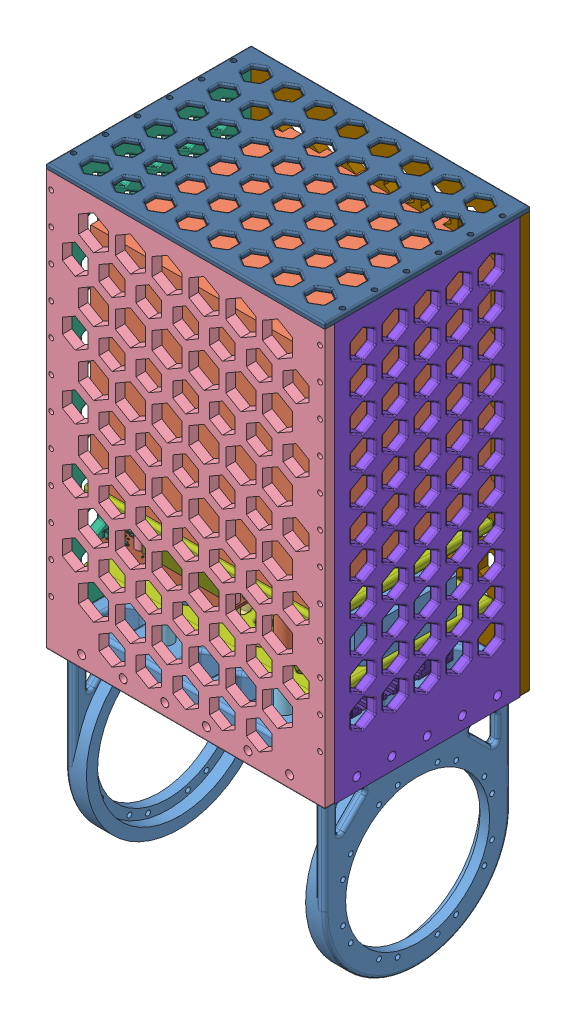
SolidWorks assembly upperbody, configuration 默认. Lengths in mm. (continued)
Components (placement in the parent): (continued)
- 交换机-1: 交换机 [默认] at (61.0275 78.8383 258.5616) x (0 0 1) z (0 -1 0) size (65.92 49.68 16.5)
  - LX-SWF502-2.step-1: LX-SWF502-2.step [Default] at (-129.5338 -11.9883 -6.5513) size (65.92 49.68 16.5)
    - RJEO-D19.step-1: RJEO-D19.step [Default] at (21.7657 41.0001 1.6) size (1.62 0.82 0.56)
      - LED0603N.step-1: LED0603N.step [Default] at origin size (1.62 0.82 0.56)
        - COMPOUND.step-1: COMPOUND.step [Default] at origin size (1.62 0.82 0.56)
    - RJEO-D2.step-1: RJEO-D2.step [Default] at (30.6411 41.0001 1.6) size (1.62 0.82 0.56)
      - LED0603N.step-1: LED0603N.step [Default] at origin size (1.62 0.82 0.56)
        - COMPOUND.step-1: COMPOUND.step [Default] at origin size (1.62 0.82 0.56)
    - RJEO-D20.step-1: RJEO-D20.step [Default] at (44.1334 41.0001 1.6) size (1.62 0.82 0.56)
      - LED0603N.step-1: LED0603N.step [Default] at origin size (1.62 0.82 0.56)
        - COMPOUND.step-1: COMPOUND.step [Default] at origin size (1.62 0.82 0.56)
    - RJEO-D21.step-1: RJEO-D21.step [Default] at (39.6501 41.0001 1.6) size (1.62 0.82 0.56)
      - LED0603N.step-1: LED0603N.step [Default] at origin size (1.62 0.82 0.56)
        - COMPOUND.step-1: COMPOUND.step [Default] at origin size (1.62 0.82 0.56)
    - RJEO-D22.step-1: RJEO-D22.step [Default] at (35.1271 41.0001 1.6) size (1.62 0.82 0.56)
      - LED0603N.step-1: LED0603N.step [Default] at origin size (1.62 0.82 0.56)
        - COMPOUND.step-1: COMPOUND.step [Default] at origin size (1.62 0.82 0.56)
    - RJEO-D1.step-1: RJEO-D1.step [Default] at (26.2147 41.0001 1.6) size (1.62 0.82 0.56)
      - LED0603N.step-1: LED0603N.step [Default] at origin size (1.62 0.82 0.56)
        - COMPOUND.step-1: COMPOUND.step [Default] at origin size (1.62 0.82 0.56)
    - RJEO-C10.step-1: RJEO-C10.step [Default] at (28.0001 37.4021 1.6) x (0 1 0) z (0 0 1) size (1 0.5 0.5)
      - 0402.step-1: 0402.step [Default] at origin size (1 0.5 0.5)
        - SOLID.step-1: SOLID.step [Default] at origin size (1 0.5 0.5)
    - RJEO-C11.step-1: RJEO-C11.step [Default] at (22.346 36.1431 1.6) x (-1 0 0) z (0 0 1) size (1 0.5 0.5)
      - 0402.step-1: 0402.step [Default] at origin size (1 0.5 0.5)
        - SOLID.step-1: SOLID.step [Default] at origin size (1 0.5 0.5)
    - RJEO-C13.step-1: RJEO-C13.step [Default] at (28.1391 26.6451 1.6) x (0 -1 0) z (0 0 1) size (1 0.5 0.5)
      - 0402.step-1: 0402.step [Default] at origin size (1 0.5 0.5)
        - SOLID.step-1: SOLID.step [Default] at origin size (1 0.5 0.5)
    - RJEO-C14.step-1: RJEO-C14.step [Default] at (32.6271 28.0611 1.6) x (0 -1 0) z (0 0 1) size (1 0.5 0.5)
      - 0402-1.step-1: 0402-1.step [Default] at origin size (1 0.5 0.5)
        - SOLID-0.step-1: SOLID-0.step [Default] at origin size (1 0.5 0.5)
    - RJEO-C15.step-1: RJEO-C15.step [Default] at (33.7611 35.9131 1.6) size (1 0.5 0.5)
      - 0402.step-1: 0402.step [Default] at origin size (1 0.5 0.5)
        - SOLID.step-1: SOLID.step [Default] at origin size (1 0.5 0.5)
    - RJEO-C16.step-1: RJEO-C16.step [Default] at (25.0001 37.5751 1.6) x (0 1 0) z (0 0 1) size (1 0.5 0.5)
      - 0402.step-1: 0402.step [Default] at origin size (1 0.5 0.5)
        - SOLID.step-1: SOLID.step [Default] at origin size (1 0.5 0.5)
    - RJEO-C17.step-1: RJEO-C17.step [Default] at (21.666 30.3191 1.6) x (-0.707107 -0.707107 0) z (0 0 1) size (1 0.5 0.5)
      - 0402.step-1: 0402.step [Default] at origin size (1 0.5 0.5)
        - SOLID.step-1: SOLID.step [Default] at origin size (1 0.5 0.5)
    - RJEO-C18.step-1: RJEO-C18.step [Default] at (23.917 26.8671 1.6) x (-0.707107 -0.707107 0) z (0 0 1) size (1 0.5 0.5)
      - 0402.step-1: 0402.step [Default] at origin size (1 0.5 0.5)
        - SOLID.step-1: SOLID.step [Default] at origin size (1 0.5 0.5)
    - RJEO-C19.step-1: RJEO-C19.step [Default] at (34.9891 39.2441 1.6) size (1 0.5 0.5)
      - 0402.step-1: 0402.step [Default] at origin size (1 0.5 0.5)
        - SOLID.step-1: SOLID.step [Default] at origin size (1 0.5 0.5)
    - RJEO-C2.step-1: RJEO-C2.step [Default] at (32.8971 20.6 1.6) x (0 1 0) z (0 0 1) size (1 0.5 0.5)
      - 0402.step-1: 0402.step [Default] at origin size (1 0.5 0.5)
        - SOLID.step-1: SOLID.step [Default] at origin size (1 0.5 0.5)
    - RJEO-C20.step-1: RJEO-C20.step [Default] at (31.5481 20.6 1.6) x (0 1 0) z (0 0 1) size (1 0.5 0.5)
      - 0402.step-1: 0402.step [Default] at origin size (1 0.5 0.5)
        - SOLID.step-1: SOLID.step [Default] at origin size (1 0.5 0.5)
    - RJEO-C25.step-1: RJEO-C25.step [Default] at (13.815 20.6 1.6) x (0 1 0) z (0 0 1) size (1 0.5 0.5)
      - 0402.step-1: 0402.step [Default] at origin size (1 0.5 0.5)
        - SOLID.step-1: SOLID.step [Default] at origin size (1 0.5 0.5)
    - RJEO-C37.step-1: RJEO-C37.step [Default] at (23.177 27.5921 1.6) x (-0.707107 -0.707107 0) z (0 0 1) size (1 0.5 0.5)
      - 0402.step-1: 0402.step [Default] at origin size (1 0.5 0.5)
        - SOLID.step-1: SOLID.step [Default] at origin size (1 0.5 0.5)
    - RJEO-C7.step-1: RJEO-C7.step [Default] at (34.7321 30.7291 1.6) x (0 -1 0) z (0 0 1) size (1 0.5 0.5)
      - 0402.step-1: 0402.step [Default] at origin size (1 0.5 0.5)
        - SOLID.step-1: SOLID.step [Default] at origin size (1 0.5 0.5)
    - RJEO-C8.step-1: RJEO-C8.step [Default] at (29.1961 26.6451 1.6) x (0 -1 0) z (0 0 1) size (1 0.5 0.5)
      - 0402.step-1: 0402.step [Default] at origin size (1 0.5 0.5)
        - SOLID.step-1: SOLID.step [Default] at origin size (1 0.5 0.5)
    - RJEO-C21.step-1: RJEO-C21.step [Default] at (5.908 27.1321 1.6) x (-1 0 0) z (0 0 1) size (1 0.5 0.5)
      - C0402.step-1: C0402.step [Default] at origin size (1 0.5 0.5)
        - SOLID-1.step-1: SOLID-1.step [Default] at origin size (1 0.5 0.5)
    - RJEO-C22.step-1: RJEO-C22.step [Default] at (6.552 21.19 1.6) size (1 0.5 0.5)
      - C0402.step-1: C0402.step [Default] at origin size (1 0.5 0.5)
        - SOLID-1.step-1: SOLID-1.step [Default] at origin size (1 0.5 0.5)
    - RJEO-C3.step-1: RJEO-C3.step [Default] at (32.5331 37.9101 1.6) x (0 1 0) z (0 0 1) size (1 0.5 0.5)
      - C0402.step-1: C0402.step [Default] at origin size (1 0.5 0.5)
        - SOLID-1.step-1: SOLID-1.step [Default] at origin size (1 0.5 0.5)
    - RJEO-C4.step-1: RJEO-C4.step [Default] at (18.817 32.7271 1.6) x (-1 0 0) z (0 0 1) size (1 0.5 0.5)
      - C0402.step-1: C0402.step [Default] at origin size (1 0.5 0.5)
        - SOLID-1.step-1: SOLID-1.step [Default] at origin size (1 0.5 0.5)
    - RJEO-C5.step-1: RJEO-C5.step [Default] at (18.81 37.8231 1.6) x (-1 0 0) z (0 0 1) size (1 0.5 0.5)
      - C0402.step-1: C0402.step [Default] at origin size (1 0.5 0.5)
        - SOLID-1.step-1: SOLID-1.step [Default] at origin size (1 0.5 0.5)
    - RJEO-C1.step-1: RJEO-C1.step [Default] at (51.3311 20.6 1.6) x (0 1 0) z (0 0 1) size (1 0.5 0.5)
      - 0402.step-1: 0402.step [Default] at origin size (1 0.5 0.5)
        - SOLID.step-1: SOLID.step [Default] at origin size (1 0.5 0.5)
    - RJEO-R11.step-1: RJEO-R11.step [Default] at (6.402 25.9921 1.6) x (-1 0 0) z (0 0 1) size (1 0.5 0.5)
      - 0402-2.step-1: 0402-2.step [Default] at origin size (1 0.5 0.5)
        - SOLID-2.step-1: SOLID-2.step [Default] at origin size (1 0.5 0.5)
    - RJEO-R12.step-1: RJEO-R12.step [Default] at (3.948 21.19 1.6) size (1 0.5 0.5)
      - 0402-2.step-1: 0402-2.step [Default] at origin size (1 0.5 0.5)
        - SOLID-2.step-1: SOLID-2.step [Default] at origin size (1 0.5 0.5)
    - RJEO-R13.step-1: RJEO-R13.step [Default] at (1.211 22.273 1.6) x (0 -1 0) z (0 0 1) size (1 0.5 0.5)
      - 0402-2.step-1: 0402-2.step [Default] at origin size (1 0.5 0.5)
        - SOLID-2.step-1: SOLID-2.step [Default] at origin size (1 0.5 0.5)
    - RJEO-R14.step-1: RJEO-R14.step [Default] at (2.295 24.326 1.6) x (0 -1 0) z (0 0 1) size (1 0.5 0.5)
      - 0402-2.step-1: 0402-2.step [Default] at origin size (1 0.5 0.5)
        - SOLID-2.step-1: SOLID-2.step [Default] at origin size (1 0.5 0.5)
    - RJEO-R15.step-1: RJEO-R15.step [Default] at (2.295 21.285 1.6) x (0 1 0) z (0 0 1) size (1 0.5 0.5)
      - 0402-2.step-1: 0402-2.step [Default] at origin size (1 0.5 0.5)
        - SOLID-2.step-1: SOLID-2.step [Default] at origin size (1 0.5 0.5)
    - RJEO-R2.step-1: RJEO-R2.step [Default] at (20.272 31.5191 1.6) size (1 0.5 0.5)
      - 0402-2.step-1: 0402-2.step [Default] at origin size (1 0.5 0.5)
        - SOLID-2.step-1: SOLID-2.step [Default] at origin size (1 0.5 0.5)
    - RJEO-R20.step-1: RJEO-R20.step [Default] at (26.4001 42.3001 1.6) size (1 0.5 0.5)
      - 0402-2.step-1: 0402-2.step [Default] at origin size (1 0.5 0.5)
        - SOLID-2.step-1: SOLID-2.step [Default] at origin size (1 0.5 0.5)
    - RJEO-R21.step-1: RJEO-R21.step [Default] at (31.0661 42.3001 1.6) size (1 0.5 0.5)
      - 0402-2.step-1: 0402-2.step [Default] at origin size (1 0.5 0.5)
        - SOLID-2.step-1: SOLID-2.step [Default] at origin size (1 0.5 0.5)
    - RJEO-R22.step-1: RJEO-R22.step [Default] at (35.6971 42.3001 1.6) size (1 0.5 0.5)
      - 0402-2.step-1: 0402-2.step [Default] at origin size (1 0.5 0.5)
        - SOLID-2.step-1: SOLID-2.step [Default] at origin size (1 0.5 0.5)
    - RJEO-R23.step-1: RJEO-R23.step [Default] at (40.2871 42.3001 1.6) size (1 0.5 0.5)
      - 0402-2.step-1: 0402-2.step [Default] at origin size (1 0.5 0.5)
        - SOLID-2.step-1: SOLID-2.step [Default] at origin size (1 0.5 0.5)
    - RJEO-R24.step-1: RJEO-R24.step [Default] at (45.0261 42.3001 1.6) size (1 0.5 0.5)
      - 0402-2.step-1: 0402-2.step [Default] at origin size (1 0.5 0.5)
        - SOLID-2.step-1: SOLID-2.step [Default] at origin size (1 0.5 0.5)
    - RJEO-R26.step-1: RJEO-R26.step [Default] at (21.524 42.3001 1.6) size (1 0.5 0.5)
      - 0402-2.step-1: 0402-2.step [Default] at origin size (1 0.5 0.5)
        - SOLID-2.step-1: SOLID-2.step [Default] at origin size (1 0.5 0.5)
    - RJEO-R3.step-1: RJEO-R3.step [Default] at (33.6221 38.4311 1.6) x (0 -1 0) z (0 0 1) size (1 0.5 0.5)
      - 0402-2.step-1: 0402-2.step [Default] at origin size (1 0.5 0.5)
        - SOLID-2.step-1: SOLID-2.step [Default] at origin size (1 0.5 0.5)
    - RJEO-R4.step-1: RJEO-R4.step [Default] at (30.3291 38.4071 1.6) x (0 -1 0) z (0 0 1) size (1 0.5 0.5)
      - 0402-2.step-1: 0402-2.step [Default] at origin size (1 0.5 0.5)
        - SOLID-2.step-1: SOLID-2.step [Default] at origin size (1 0.5 0.5)
    - RJEO-R5.step-1: RJEO-R5.step [Default] at (44.0581 42.3001 1.6) x (-1 0 0) z (0 0 1) size (1 0.5 0.5)
      - 0402-2.step-1: 0402-2.step [Default] at origin size (1 0.5 0.5)
        - SOLID-2.step-1: SOLID-2.step [Default] at origin size (1 0.5 0.5)
    - RJEO-R6.step-1: RJEO-R6.step [Default] at (39.2791 42.3001 1.6) x (-1 0 0) z (0 0 1) size (1 0.5 0.5)
      - 0402-2.step-1: 0402-2.step [Default] at origin size (1 0.5 0.5)
        - SOLID-2.step-1: SOLID-2.step [Default] at origin size (1 0.5 0.5)
    - RJEO-R7.step-1: RJEO-R7.step [Default] at (34.6091 42.3001 1.6) x (-1 0 0) z (0 0 1) size (1 0.5 0.5)
      - 0402-2.step-1: 0402-2.step [Default] at origin size (1 0.5 0.5)
        - SOLID-2.step-1: SOLID-2.step [Default] at origin size (1 0.5 0.5)
    - RJEO-R8.step-1: RJEO-R8.step [Default] at (30.0421 42.3001 1.6) x (-1 0 0) z (0 0 1) size (1 0.5 0.5)
      - 0402-2.step-1: 0402-2.step [Default] at origin size (1 0.5 0.5)
        - SOLID-2.step-1: SOLID-2.step [Default] at origin size (1 0.5 0.5)
    - RJEO-R9.step-1: RJEO-R9.step [Default] at (25.3031 42.3001 1.6) x (-1 0 0) z (0 0 1) size (1 0.5 0.5)
      - 0402-2.step-1: 0402-2.step [Default] at origin size (1 0.5 0.5)
        - SOLID-2.step-1: SOLID-2.step [Default] at origin size (1 0.5 0.5)
    - RJEO-R1.step-1: RJEO-R1.step [Default] at (31.4191 37.4141 1.6) x (0 1 0) z (0 0 1) size (1 0.5 0.5)
      - 0402-2.step-1: 0402-2.step [Default] at origin size (1 0.5 0.5)
        - SOLID-2.step-1: SOLID-2.step [Default] at origin size (1 0.5 0.5)
    - RJEO-JP1.step-1: RJEO-JP1.step [Default] at (12.001 40.0001 1.6) x (-1 0 0) z (0 0 1) size (7.5 5.9 10.6)
      - SIP2.step-1: SIP2.step [Default] at origin size (7.5 5.9 10.6)
        - COMPOUND-3.step-1: COMPOUND-3.step [Default] at origin size (7.5 5.9 10.6)
    - RJEO-DXFRM3.step-1: RJEO-DXFRM3.step [Default] at (21.989 19.3 1.6) x (-1 0 0) z (0 0 1) size (15.1 10 4.5)
      - NS892407B.step-1: NS892407B.step [Default] at origin size (15.1 10 4.5)
        - COMPOUND-4.step-1: COMPOUND-4.step [Default] at origin size (15.1 10 4.5)
    - RJEO-DXFRM1.step-1: RJEO-DXFRM1.step [Default] at (41.7141 19.3 1.6) x (-1 0 0) z (0 0 1) size (15.1 10 4.5)
      - NS892407B.step-1: NS892407B.step [Default] at origin size (15.1 10 4.5)
        - COMPOUND-4.step-1: COMPOUND-4.step [Default] at origin size (15.1 10 4.5)
    - RJEO-L2.step-1: RJEO-L2.step [Default] at (10.114 25.031 1.6) x (0 -1 0) z (0 0 1) size (4.4 4.2 2.1)
      - L10A.step-1: L10A.step [Default] at origin size (4.4 4.2 2.1)
        - SOLID-5.step-1: SOLID-5.step [Default] at origin size (4.4 4.2 2.1)
    - RJEO-TC4.step-1: RJEO-TC4.step [Default] at (4.629 32.6291 1.6) x (0 -1 0) z (0 0 1) size (6.6 7.8 7.75)
      - CAP-E-SMD-D6.3.step-1: CAP-E-SMD-D6.3.step [Default] at origin size (6.6 7.8 7.75)
        - SOLID-6.step-1: SOLID-6.step [Default] at origin size (6.6 7.8 7.75)
    - RJEO-TC1.step-1: RJEO-TC1.step [Default] at (16 28.8001 1.6) x (0 1 0) z (0 0 1) size (6.6 7.8 7.75)
      - CAP-E-SMD-D6.3.step-1: CAP-E-SMD-D6.3.step [Default] at origin size (6.6 7.8 7.75)
        - SOLID-6.step-1: SOLID-6.step [Default] at origin size (6.6 7.8 7.75)
    - RJEO-TRS1.step-1: RJEO-TRS1.step [Default] at (41.5201 33.5001 1.6) x (0 -1 0) z (0 0 1) size (12.7 9.5 5.95)
      - RJ45-8PIN.step-1: RJ45-8PIN.step [Default] at origin size (12.7 9.5 5.95)
        - COMPOUND-7.step-1: COMPOUND-7.step [Default] at origin size (12.7 9.5 5.95)
    - RJEO-Y6.step-1: RJEO-Y6.step [Default] at (18.772 35.3521 1.6) x (0 1 0) z (0 0 1) size (3.2 2.5 0.72)
      - SM091.step-1: SM091.step [Default] at origin size (3.2 2.5 0.72)
        - SOLID-8.step-1: SOLID-8.step [Default] at origin size (3.2 2.5 0.72)
    - RJEO-U1.step-1: RJEO-U1.step [Default] at (6.457 22.482 1.6) x (0 1 0) z (0 0 1) size (2.88 2.79 1.64)
      - SOT23-6.step-1: SOT23-6.step [Default] at origin size (2.88 2.79 1.64)
        - COMPOUND-9.step-1: COMPOUND-9.step [Default] at origin size (2.88 2.79 1.64)
    - RJEO-U2.step-1: RJEO-U2.step [Default] at (28.0001 32.0001 1.6) x (-1 0 0) z (0 0 1) size (6 6 0.85)
      - QFN48_04_EPAD.step-1: QFN48_04_EPAD.step [Default] at origin size (6 6 0.85)
        - COMPOUND-10.step-1: COMPOUND-10.step [Default] at origin size (6 6 0.85)
    - RJEO-H6.step-1: RJEO-H6.step [Default] at (56.8961 40.8691 1.6) x (-1 0 0) z (0 0 1) size (16.45 16.05 15.8)
      - RJ45-1X1-B.step-1: RJ45-1X1-B.step [Default] at origin size (16.45 16.05 15.8)
        - COMPOUND-11.step-1: COMPOUND-11.step [Default] at origin size (16.45 16.05 15.8)
    - RJEO-H7.step-1: RJEO-H7.step [Default] at (33.1521 2.093 1.6) size (63.76 15.76 16.2)
      - RJ45-1X4-B.step-1: RJ45-1X4-B.step [Default] at origin size (63.76 15.76 16.2)
        - COMPOUND-12.step-1: COMPOUND-12.step [Default] at origin size (63.76 15.76 16.2)
    - Board.step-1: Board.step [Default] at origin size (65.92 43.41 1.6)
- 转压-1: 转压 [默认] at (54.0084 99.9888 161.9625) x (-1 0 0) z (0 0 -1) size (57.6 22 63.7)
- ctrlbox-3: ctrlbox [默认] at (5.0084 130.5588 162) size (148 6 110)
- M6螺柱35-3: M6螺柱35 [默认] at (42.5084 93.9888 122) x (0.932693 0 -0.360672) z (0.360672 0 0.932693) size (10 35 10)
- M6螺柱35-4: M6螺柱35 [默认] at (42.5084 93.9888 202) x (0.513313 0 -0.858202) z (0.858202 0 0.513313) size (10 35 10)
- M3螺柱10-5: M3螺柱10 [默认] at (10.5084 93.9888 116) size (6 10 6)
- M3螺柱10-6: M3螺柱10 [默认] at (-47.4916 93.9888 116) size (6 10 6)
- M3螺柱10-7: M3螺柱10 [默认] at (-47.4916 93.9888 202) size (6 10 6)
- M3螺柱10-8: M3螺柱10 [默认] at (10.5084 93.9888 202) size (6 10 6)
- M3螺柱25-1: M3螺柱25 [默认] at (10.5084 105.5588 116) x (0.994103 0 0.108442) z (-0.108442 0 0.994103) size (6 25 6)
- M3螺柱25-2: M3螺柱25 [默认] at (-47.4916 105.5588 116) x (0.999732 0 0.023161) z (-0.023161 0 0.999732) size (6 25 6)
- M3螺柱25-3: M3螺柱25 [默认] at (-47.4916 105.5588 202) x (0.999732 0 0.023161) z (-0.023161 0 0.999732) size (6 25 6)
- M3螺柱25-4: M3螺柱25 [默认] at (10.5084 105.5588 202) x (0.999732 0 0.023161) z (-0.023161 0 0.999732) size (6 25 6)
- M4螺柱6-1: M4螺柱6 [默认] at (51.5084 93.9888 188.9625) x (0.999997 0 -0.002414) z (0.002414 0 0.999997) size (6 6 6)
- M4螺柱6-2: M4螺柱6 [默认] at (51.5084 93.9888 134.9625) x (0.9996 0 -0.02829) z (0.02829 0 0.9996) size (6 6 6)
Mates (geometry in assembly coordinates):
- Coincident1: coincident anti-aligned: plane of crotch-1 through (85.5084 62.9888 162) normal (0 1 0); plane of imu-1 through (4.5084 62.9888 136) normal (0 -1 0)
- Concentric1: concentric anti-aligned: cylinder of crotch-1 through (4.5084 42.9888 116.5) axis (0 1 0) radius 1.5; cylinder of imu-1 through (4.5084 66.9888 116.5) axis (0 -1 0) radius 1.6
- Concentric2: concentric anti-aligned: cylinder of crotch-1 through (-12.4916 42.9888 155.5) axis (0 1 0) radius 1.5; cylinder of imu-1 through (-12.4916 66.9888 155.5) axis (0 -1 0) radius 1.6
- Coincident4: coincident anti-aligned: plane of crotch-1 through (85.5084 -17.0112 220) normal (0 0 1); plane of front-1 through (4.5084 194.9888 220) normal (0 0 -1)
- Concentric3: concentric aligned: cylinder of crotch-1 through (-60.4916 52.9888 213) axis (0 0 1) radius 2.5; cylinder of front-1 through (-60.4916 52.9888 220) axis (0 0 1) radius 2.5
- Concentric4: concentric aligned: cylinder of crotch-1 through (69.5084 52.9888 213) axis (0 0 1) radius 2.5; cylinder of front-1 through (69.5084 52.9888 220) axis (0 0 1) radius 2.5
- Concentric5: concentric anti-aligned: cylinder of crotch-1 through (42.5084 42.9888 122) axis (0 1 0) radius 3; cylinder of M8螺柱-1 through (42.5084 87.9888 122) axis (0 -1 0) radius 3
- Coincident6: coincident anti-aligned: plane of crotch-1 through (85.5084 62.9888 162) normal (0 1 0); plane of M8螺柱-1 through (42.5084 62.9888 122) normal (0 -1 0)
- Concentric6: concentric anti-aligned: cylinder of crotch-1 through (42.5084 42.9888 202) axis (0 1 0) radius 3; cylinder of M8螺柱-2 through (42.5084 87.9888 202) axis (0 -1 0) radius 3
- Coincident7: coincident anti-aligned: plane of crotch-1 through (85.5084 62.9888 162) normal (0 1 0); plane of M8螺柱-2 through (42.5084 62.9888 202) normal (0 -1 0)
- Concentric7: concentric anti-aligned: cylinder of crotch-1 through (-32.4916 42.9888 122) axis (0 1 0) radius 3; cylinder of M8螺柱-3 through (-32.4916 87.9888 122) axis (0 -1 0) radius 3
- Coincident8: coincident anti-aligned: plane of crotch-1 through (85.5084 62.9888 162) normal (0 1 0); plane of M8螺柱-3 through (-32.4916 62.9888 122) normal (0 -1 0)
- Concentric8: concentric anti-aligned: cylinder of crotch-1 through (-32.4916 42.9888 202) axis (0 1 0) radius 3; cylinder of M8螺柱-4 through (-32.4916 87.9888 202) axis (0 -1 0) radius 5
- Coincident9: coincident anti-aligned: plane of crotch-1 through (85.5084 62.9888 162) normal (0 1 0); plane of M8螺柱-4 through (-32.4916 62.9888 202) normal (0 -1 0)
- Concentric9: concentric anti-aligned: cylinder of crotch-1 through (-69.4916 52.9888 184) axis (-1 0 0) radius 2.5; cylinder of left-1 through (-82.4916 52.9888 184) axis (1 0 0) radius 2.5
- Concentric10: concentric anti-aligned: cylinder of crotch-1 through (-69.4916 52.9888 140) axis (-1 0 0) radius 2.5; cylinder of left-1 through (-82.4916 52.9888 140) axis (1 0 0) radius 2.5
- Coincident10: coincident anti-aligned: plane of crotch-1 through (-76.4916 -17.0112 162) normal (-1 0 0); plane of left-1 through (-76.4916 204.9888 162) normal (1 0 0)
- Concentric11: concentric anti-aligned: cylinder of crotch-1 through (78.5084 52.9888 118) axis (1 0 0) radius 2.5; cylinder of right-1 through (91.5084 52.9888 118) axis (-1 0 0) radius 2.5
- Concentric12: concentric anti-aligned: cylinder of crotch-1 through (78.5084 52.9888 206) axis (1 0 0) radius 2.5; cylinder of right-1 through (91.5084 52.9888 206) axis (-1 0 0) radius 2.5
- Coincident11: coincident anti-aligned: plane of crotch-1 through (85.5084 -17.0112 162) normal (1 0 0); plane of right-1 through (85.5084 204.9888 162) normal (-1 0 0)
- Concentric13: concentric anti-aligned: cylinder of M8螺柱-1 through (42.5084 87.9888 122) axis (0 -1 0) radius 3; cylinder of ctrlbox-2 through (42.5084 87.9888 122) axis (0 1 0) radius 3
- Concentric14: concentric anti-aligned: cylinder of M8螺柱-4 through (-32.4916 87.9888 202) axis (0 -1 0) radius 3; cylinder of ctrlbox-2 through (-32.4916 87.9888 202) axis (0 1 0) radius 3
- Coincident13: coincident anti-aligned: plane of M8螺柱-3 through (-32.4916 87.9888 122) normal (0 1 0); plane of ctrlbox-2 through (5.0084 87.9888 162) normal (0 -1 0)
- Concentric22: concentric anti-aligned: cylinder of crotch-1 through (69.5084 52.9888 111) axis (0 0 -1) radius 2.5; cylinder of back-2 through (69.5084 52.9888 98) axis (0 0 1) radius 2.5
- Concentric23: concentric anti-aligned: cylinder of crotch-1 through (-60.4916 52.9888 111) axis (0 0 -1) radius 2.5; cylinder of back-2 through (-60.4916 52.9888 98) axis (0 0 1) radius 2.5
- Coincident22: coincident anti-aligned: plane of crotch-1 through (85.5084 -17.0112 104) normal (0 0 -1); plane of back-2 through (4.5084 194.9888 104) normal (0 0 1)
- Concentric39: concentric aligned: cylinder of right-1 through (88.5084 296.9888 212) axis (0 1 0) radius 1.5; cylinder of top-1 through (88.5084 304.9888 212) axis (0 1 0) radius 1.5
- Concentric40: concentric aligned: cylinder of left-1 through (-79.4916 296.9888 212) axis (0 1 0) radius 1.5; cylinder of top-1 through (-79.4916 304.9888 212) axis (0 1 0) radius 1.5
- Coincident26: coincident anti-aligned: plane of front-1 through (4.5084 304.9888 220) normal (0 1 0); plane of top-1 through (4.5084 304.9888 162) normal (0 -1 0)
- Parallel11: parallel anti-aligned: plane of battery-1 through (73.2915 136.5588 99.1011) normal (0 -1 0); plane of ctrlbox-2 through (5.0084 93.9888 162) normal (0 1 0)
- Parallel12: parallel aligned: plane of crotch-1 through (85.5084 -17.0112 104) normal (0 0 -1); plane of battery-1 through (3.2915 206.5588 99.1011) normal (0 0 -1)
- Concentric44: concentric aligned: cylinder of ctrlbox-2 through (10.5084 83.9888 202) axis (0 1 0) radius 1.5; cylinder of jetsonnano-1/675_13541_batuu_dev_kit_top_ass_asm.stp-1/642-13541_BATUU_SYS_BOM_ASM.stp-1/600-13542-BASE-A02_ASM.stp-1/600-13542-BASE-A02.stp-1 through (10.5084 103.9888 202) axis (0 1 0) radius 1.375
- Concentric45: concentric aligned: cylinder of ctrlbox-2 through (10.5084 83.9888 116) axis (0 1 0) radius 1.5; cylinder of jetsonnano-1/675_13541_batuu_dev_kit_top_ass_asm.stp-1/642-13541_BATUU_SYS_BOM_ASM.stp-1/600-13542-BASE-A02_ASM.stp-1/600-13542-BASE-A02.stp-1 through (10.5084 103.9888 116) axis (0 1 0) radius 1.375
- Concentric62: concentric aligned: cylinder of ctrlbox-2 through (46.7384 83.9888 192.09) axis (0 1 0) radius 1.5; cylinder of 交换机-1/LX-SWF502-2.step-1/Board.step-1 through (46.7384 85.3897 192.09) axis (0 1 0) radius 1.5
- Parallel17: parallel aligned: plane of ctrlbox-2 through (-68.9916 93.9888 217) normal (0 0 1); plane of 交换机-1/LX-SWF502-2.step-1/Board.step-1 through (29.7887 85.3897 194.9996) normal (0 0 1)
- Parallel18: parallel aligned: plane of ctrlbox-2 through (79.0084 93.9888 217) normal (1 0 0); plane of 交换机-1/LX-SWF502-2.step-1/Board.step-1 through (73.202 85.3897 194.9996) normal (1 0 0)
- Parallel19: parallel anti-aligned: plane of ctrlbox-2 through (5.0084 93.9888 162) normal (0 1 0); plane of 转压-1 through (54.0084 99.9888 161.9625) normal (0 -1 0)
- Parallel20: parallel aligned: plane of ctrlbox-2 through (79.0084 93.9888 217) normal (1 0 0); plane of 转压-1 through (82.8084 121.9888 188.8125) normal (1 0 0)
- Coincident45: coincident anti-aligned: plane of battery-1 through (73.2915 136.5588 99.1011) normal (0 -1 0); plane of ctrlbox-3 through (5.0084 136.5588 162) normal (0 1 0)
- Concentric69: concentric anti-aligned: cylinder of ctrlbox-2 through (42.5084 87.9888 122) axis (0 1 0) radius 3; cylinder of M6螺柱35-3 through (42.5084 128.9888 122) axis (0 -1 0) radius 3
- Coincident46: coincident anti-aligned: plane of ctrlbox-2 through (5.0084 93.9888 162) normal (0 1 0); plane of M6螺柱35-3 through (42.5084 93.9888 122) normal (0 -1 0)
- Concentric70: concentric anti-aligned: cylinder of ctrlbox-2 through (42.5084 87.9888 202) axis (0 1 0) radius 3; cylinder of M6螺柱35-4 through (42.5084 128.9888 202) axis (0 -1 0) radius 3
- Coincident47: coincident anti-aligned: plane of ctrlbox-2 through (5.0084 93.9888 162) normal (0 1 0); plane of M6螺柱35-4 through (42.5084 93.9888 202) normal (0 -1 0)
- Concentric71: concentric anti-aligned: cylinder of jetsonnano-1/675_13541_batuu_dev_kit_top_ass_asm.stp-1/642-13541_BATUU_SYS_BOM_ASM.stp-1/600-13542-BASE-A02_ASM.stp-1/600-13542-BASE-A02.stp-1 through (10.5084 103.9888 116) axis (0 1 0) radius 1.375; cylinder of M3螺柱10-5 through (10.5084 103.9888 116) axis (0 -1 0) radius 1.5
- Coincident48: coincident anti-aligned: plane of ctrlbox-2 through (5.0084 93.9888 162) normal (0 1 0); plane of M3螺柱10-5 through (10.5084 93.9888 116) normal (0 -1 0)
- Coincident49: coincident anti-aligned: plane of jetsonnano-1/675_13541_batuu_dev_kit_top_ass_asm.stp-1/642-13541_BATUU_SYS_BOM_ASM.stp-1/600-13542-BASE-A02_ASM.stp-1/600-13542-BASE-A02.stp-1 through (-47.4916 103.9888 116) normal (0 -1 0); plane of M3螺柱10-5 through (10.5084 103.9888 116) normal (0 1 0)
- Concentric72: concentric anti-aligned: cylinder of ctrlbox-2 through (-47.4916 83.9888 116) axis (0 1 0) radius 1.5; cylinder of M3螺柱10-6 through (-47.4916 103.9888 116) axis (0 -1 0) radius 1.5
- Coincident50: coincident anti-aligned: plane of jetsonnano-1/675_13541_batuu_dev_kit_top_ass_asm.stp-1/642-13541_BATUU_SYS_BOM_ASM.stp-1/600-13542-BASE-A02_ASM.stp-1/600-13542-BASE-A02.stp-1 through (-47.4916 103.9888 116) normal (0 -1 0); plane of M3螺柱10-6 through (-47.4916 103.9888 116) normal (0 1 0)
- Concentric73: concentric anti-aligned: cylinder of jetsonnano-1/675_13541_batuu_dev_kit_top_ass_asm.stp-1/642-13541_BATUU_SYS_BOM_ASM.stp-1/600-13542-BASE-A02_ASM.stp-1/600-13542-BASE-A02.stp-1 through (-47.4916 103.9888 202) axis (0 1 0) radius 1.375; cylinder of M3螺柱10-7 through (-47.4916 103.9888 202) axis (0 -1 0) radius 1.5
- Coincident51: coincident anti-aligned: plane of ctrlbox-2 through (5.0084 93.9888 162) normal (0 1 0); plane of M3螺柱10-7 through (-47.4916 93.9888 202) normal (0 -1 0)
- Concentric74: concentric anti-aligned: cylinder of jetsonnano-1/675_13541_batuu_dev_kit_top_ass_asm.stp-1/642-13541_BATUU_SYS_BOM_ASM.stp-1/600-13542-BASE-A02_ASM.stp-1/600-13542-BASE-A02.stp-1 through (10.5084 103.9888 202) axis (0 1 0) radius 1.375; cylinder of M3螺柱10-8 through (10.5084 103.9888 202) axis (0 -1 0) radius 1.5
- Coincident52: coincident anti-aligned: plane of jetsonnano-1/675_13541_batuu_dev_kit_top_ass_asm.stp-1/642-13541_BATUU_SYS_BOM_ASM.stp-1/600-13542-BASE-A02_ASM.stp-1/600-13542-BASE-A02.stp-1 through (-47.4916 103.9888 116) normal (0 -1 0); plane of M3螺柱10-8 through (10.5084 103.9888 202) normal (0 1 0)
- Concentric75: concentric anti-aligned: cylinder of jetsonnano-1/675_13541_batuu_dev_kit_top_ass_asm.stp-1/642-13541_BATUU_SYS_BOM_ASM.stp-1/600-13542-BASE-A02_ASM.stp-1/600-13542-BASE-A02.stp-1 through (10.5084 103.9888 116) axis (0 1 0) radius 1.375; cylinder of M3螺柱25-1 through (10.5084 130.5588 116) axis (0 -1 0) radius 1.5
- Coincident53: coincident anti-aligned: plane of jetsonnano-1/675_13541_batuu_dev_kit_top_ass_asm.stp-1/642-13541_BATUU_SYS_BOM_ASM.stp-1/600-13542-BASE-A02_ASM.stp-1/600-13542-BASE-A02.stp-1 through (-47.4916 105.5588 116) normal (0 1 0); plane of M3螺柱25-1 through (10.5084 105.5588 116) normal (0 -1 0)
- Concentric76: concentric anti-aligned: cylinder of jetsonnano-1/675_13541_batuu_dev_kit_top_ass_asm.stp-1/642-13541_BATUU_SYS_BOM_ASM.stp-1/600-13542-BASE-A02_ASM.stp-1/600-13542-BASE-A02.stp-1 through (-47.4916 103.9888 116) axis (0 1 0) radius 1.375; cylinder of M3螺柱25-2 through (-47.4916 130.5588 116) axis (0 -1 0) radius 1.5
- Coincident54: coincident anti-aligned: plane of jetsonnano-1/675_13541_batuu_dev_kit_top_ass_asm.stp-1/642-13541_BATUU_SYS_BOM_ASM.stp-1/600-13542-BASE-A02_ASM.stp-1/600-13542-BASE-A02.stp-1 through (-47.4916 105.5588 116) normal (0 1 0); plane of M3螺柱25-2 through (-47.4916 105.5588 116) normal (0 -1 0)
- Concentric77: concentric anti-aligned: cylinder of jetsonnano-1/675_13541_batuu_dev_kit_top_ass_asm.stp-1/642-13541_BATUU_SYS_BOM_ASM.stp-1/600-13542-BASE-A02_ASM.stp-1/600-13542-BASE-A02.stp-1 through (-47.4916 103.9888 202) axis (0 1 0) radius 1.375; cylinder of M3螺柱25-3 through (-47.4916 130.5588 202) axis (0 -1 0) radius 1.5
- Coincident55: coincident anti-aligned: plane of ctrlbox-3 through (5.0084 130.5588 162) normal (0 -1 0); plane of M3螺柱25-3 through (-47.4916 130.5588 202) normal (0 1 0)
- Coincident56: coincident anti-aligned: plane of jetsonnano-1/675_13541_batuu_dev_kit_top_ass_asm.stp-1/642-13541_BATUU_SYS_BOM_ASM.stp-1/600-13542-BASE-A02_ASM.stp-1/600-13542-BASE-A02.stp-1 through (-47.4916 105.5588 116) normal (0 1 0); plane of M3螺柱25-3 through (-47.4916 105.5588 202) normal (0 -1 0)
- Concentric78: concentric anti-aligned: cylinder of jetsonnano-1/675_13541_batuu_dev_kit_top_ass_asm.stp-1/642-13541_BATUU_SYS_BOM_ASM.stp-1/600-13542-BASE-A02_ASM.stp-1/600-13542-BASE-A02.stp-1 through (10.5084 103.9888 202) axis (0 1 0) radius 1.375; cylinder of M3螺柱25-4 through (10.5084 130.5588 202) axis (0 -1 0) radius 1.5
- Coincident57: coincident anti-aligned: plane of ctrlbox-3 through (5.0084 130.5588 162) normal (0 -1 0); plane of M3螺柱25-4 through (10.5084 130.5588 202) normal (0 1 0)
- Concentric79: concentric anti-aligned: cylinder of ctrlbox-3 through (-47.4916 126.5588 116) axis (0 1 0) radius 1.5; cylinder of M3螺柱25-2 through (-47.4916 130.5588 116) axis (0 -1 0) radius 1.5
- Concentric80: concentric anti-aligned: cylinder of ctrlbox-3 through (-47.4916 126.5588 202) axis (0 1 0) radius 1.5; cylinder of M3螺柱25-3 through (-47.4916 130.5588 202) axis (0 -1 0) radius 1.5
- Coincident58: coincident anti-aligned: plane of battery-1 through (73.2915 136.5588 99.1011) normal (0 -1 0); plane of ctrlbox-3 through (5.0084 136.5588 162) normal (0 1 0)
- Concentric81: concentric anti-aligned: cylinder of ctrlbox-2 through (51.5084 83.9888 188.9625) axis (0 1 0) radius 2; cylinder of 转压-1 through (51.5084 121.9888 188.9625) axis (0 -1 0) radius 3.25
- Concentric82: concentric anti-aligned: cylinder of ctrlbox-2 through (51.5084 83.9888 134.9625) axis (0 1 0) radius 2; cylinder of 转压-1 through (51.5084 121.9888 134.9625) axis (0 -1 0) radius 3.25
- Concentric83: concentric anti-aligned: cylinder of ctrlbox-2 through (51.5084 83.9888 188.9625) axis (0 1 0) radius 2; cylinder of M4螺柱6 - 副本-1 through (51.5084 99.9888 188.9625) axis (0 -1 0) radius 2
- Coincident59: coincident anti-aligned: plane of ctrlbox-2 through (5.0084 93.9888 162) normal (0 1 0); plane of M4螺柱6 - 副本-1 through (51.5084 93.9888 188.9625) normal (0 -1 0)
- Coincident60: coincident anti-aligned: plane of 转压-1 through (54.0084 99.9888 161.9625) normal (0 -1 0); plane of M4螺柱6 - 副本-1 through (51.5084 99.9888 188.9625) normal (0 1 0)
- Concentric84: concentric aligned: cylinder of 转压-1 through (51.5084 121.9888 134.9625) axis (0 -1 0) radius 3.25; cylinder of M4螺柱6 - 副本-2 through (51.5084 99.9888 134.9625) axis (0 -1 0) radius 2
- Coincident61: coincident anti-aligned: plane of ctrlbox-2 through (5.0084 93.9888 162) normal (0 1 0); plane of M4螺柱6 - 副本-2 through (51.5084 93.9888 134.9625) normal (0 -1 0)
